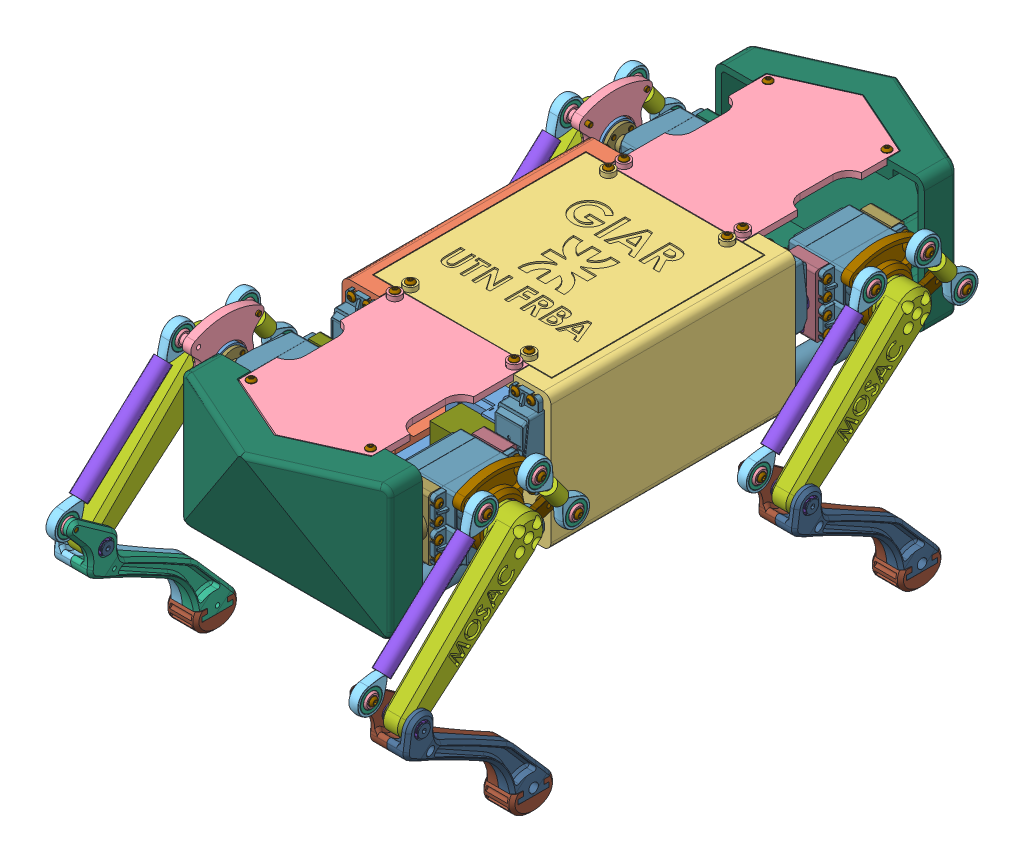
SolidWorks assembly Cuerpo_completo, configuration Default. Lengths in mm. (continued)
Components (placement in the parent): (continued)
- NUCLEO-F412ZG-3: NUCLEO-F412ZG [Default] at (0 3.6 5.7301) size (70 15.53 135.45)
- PCB_Interconexion-2: PCB_Interconexion [Default] at (-47.75 25.1914 50) x (1 0 0) z (0 1 0) size (106 111.32 17.03)
- IDC_40-1: IDC_40 [Default] at (-39.1382 -11.973 -4.2522) x (0 0 -1) z (1 0 0) size (55.48 10.75 7.86) (hidden)
- IDC_50-1: IDC_50 [Default] at (-15.8418 7.607 14.5537) x (0 0 1) z (-1 0 0) size (68.18 10.75 7.86) (hidden)
- IDC_50-2: IDC_50 [Default] at (45.1182 7.607 14.5537) x (0 0 1) z (-1 0 0) size (68.18 10.75 7.86) (hidden)
- IDC_50-4: IDC_50 [Default] at (4.87 250.7726 68.2196) x (0 0 -1) z (1 0 0) size (68.18 10.75 7.86) (hidden)
- IDC_50-5: IDC_50 [Default] at (-13.5299 250.7726 68.2196) x (0 0 -1) z (1 0 0) size (68.18 10.75 7.86) (hidden)
- IDC_40-2: IDC_40 [Default] at (-37.9534 250.7726 87.0269) x (0 0 1) z (-1 0 0) size (55.48 10.75 7.86) (hidden)
- USB-A-1: USB-A [Default] at (-40.9616 252.3756 123.8231) x (-1 0 0) z (0 0 -1) size (15 7 40) (hidden)
- USB-C-1: USB-C [Default] at (-43.6584 -12.82 23.9114) x (0 0 1) z (-1 0 0) size (10 5 29) (hidden)
- USB-C_90_Degree-1: USB-C_90_Degree [Default] at (31.45 -12.82 23.9114) x (0 0 -1) z (-1 0 0) size (25.07 7.5 16.55) (hidden)
- Tapa-1: Tapa [Default] at (0 39.5 0) size (114.5 7 136.5)
- Tapa_extrema-3: Tapa_extrema [Default] at (0 39.5 -161.6) x (1 0 0) z (0 1 0) size (85.5 120.4 7)
- Tapa_extrema-4: Tapa_extrema [Default] at (0.3648 39.5 161.4403) x (-0.999991 0 0.004156) z (0 1 0) size (85.5 120.4 7)
- Tornillo_boton_M3-1: Tornillo_boton_M3 [12] at (57.75 37.95 83.4927) x (0 0 -1) z (-1 -0.000079 0) size (13.65 5.5 5.5)
- Tornillo_boton_M3-2: Tornillo_boton_M3 [12] at (47.75 37.95 83.4927) x (0 0 -1) z (-0.987363 0.158475 0) size (13.65 5.5 5.5)
- Tornillo_boton_M3-4: Tornillo_boton_M3 [12] at (57.75 37.95 -83.4927) x (0 0 1) z (-0.423407 0.90594 0) size (13.65 5.5 5.5)
- Tornillo_boton_M3-6: Tornillo_boton_M3 [12] at (47.75 37.95 -83.4927) x (0 0 1) z (-0.25966 0.9657 0) size (13.65 5.5 5.5)
- Tornillo_boton_M3-8: Tornillo_boton_M3 [12] at (57.75 -11.55 83.4927) x (0 0 -1) z (-0.907023 0.421082 0) size (13.65 5.5 5.5)
- Tornillo_boton_M3-10: Tornillo_boton_M3 [12] at (47.75 -11.55 83.4927) x (0 0 -1) z (-0.902883 0.429885 0) size (13.65 5.5 5.5)
- Tornillo_boton_M3-12: Tornillo_boton_M3 [12] at (47.75 -11.55 -83.4927) x (0 0 1) z (0.257978 0.966151 0) size (13.65 5.5 5.5)
- Tornillo_boton_M3-14: Tornillo_boton_M3 [12] at (57.75 -11.55 -83.4927) x (0 0 1) z (0.421829 0.906675 0) size (13.65 5.5 5.5)
- Tornillo_boton_M3-16: Tornillo_boton_M3 [12] at (-47.75 -11.55 -83.4927) x (0 0 1) z (0.572863 0.819651 0) size (13.65 5.5 5.5)
- Tornillo_boton_M3-18: Tornillo_boton_M3 [12] at (-57.75 -11.55 -83.4927) x (0 0 1) z (0.706491 0.707722 0) size (13.65 5.5 5.5)
- Tornillo_boton_M3-20: Tornillo_boton_M3 [12] at (-47.75 37.95 -83.4927) x (0 0 1) z (0.818652 0.574289 0) size (13.65 5.5 5.5)
- Tornillo_boton_M3-22: Tornillo_boton_M3 [12] at (-57.75 37.95 -83.4927) x (0 0 1) z (0.90594 0.423407 0) size (13.65 5.5 5.5)
- Tornillo_boton_M3-24: Tornillo_boton_M3 [12] at (-47.75 37.95 83.4927) x (0 0 -1) z (-0.919584 -0.392893 0) size (13.65 5.5 5.5)
- Tornillo_boton_M3-26: Tornillo_boton_M3 [12] at (-57.75 37.95 83.4927) x (0 0 -1) z (-0.902816 -0.430028 0) size (13.65 5.5 5.5)
- Tornillo_boton_M3-28: Tornillo_boton_M3 [12] at (-47.75 -11.55 83.4927) x (0 0 -1) z (-0.906956 -0.421225 0) size (13.65 5.5 5.5)
- Tornillo_boton_M3-30: Tornillo_boton_M3 [12] at (-57.75 -11.55 83.4927) x (0 0 -1) z (-0.928542 -0.371227 0) size (13.65 5.5 5.5)
- Tornillo_boton_M3-31: Tornillo_boton_M3 [12] at (38.25 48.15 -63.75) x (0 -1 0) z (0.000424 0 1) size (13.65 5.5 5.5)
- Tornillo_boton_M3-32: Tornillo_boton_M3 [12] at (38.25 48.15 -73.75) x (0 -1 0) z (0.188872 0 0.982002) size (13.65 5.5 5.5)
- Tornillo_boton_M3-33: Tornillo_boton_M3 [12] at (-38.25 48.15 -63.75) x (0 -1 0) z (0.188872 0 0.982002) size (13.65 5.5 5.5)
- Tornillo_boton_M3-35: Tornillo_boton_M3 [12] at (-38.25 48.15 -73.75) x (0 -1 0) z (0.396124 0 0.918197) size (13.65 5.5 5.5)
- Tornillo_boton_M3-37: Tornillo_boton_M3 [12] at (-38.25 48.15 63.75) x (0 -1 0) z (0.600339 0 0.799745) size (13.65 5.5 5.5)
- Tornillo_boton_M3-39: Tornillo_boton_M3 [12] at (38.25 48.15 63.75) x (0 -1 0) z (0.773946 0 0.633251) size (13.65 5.5 5.5)
- Tornillo_boton_M3-41: Tornillo_boton_M3 [12] at (38.2493 48.15 73.4321) x (0 -1 0) z (0.896399 0 0.443249) size (13.65 5.5 5.5)
- Tornillo_boton_M3-43: Tornillo_boton_M3 [12] at (-38.25 48.15 73.75) x (0 -1 0) z (0.964846 0 0.262815) size (13.65 5.5 5.5)
- Tornillo_boton_M3-44: Tornillo_boton_M3 [12] at (-37.8641 45.15 166.5992) x (0 -1 0) z (0.997087 0 0.076276) size (13.65 5.5 5.5)
- Tornillo_boton_M3-46: Tornillo_boton_M3 [12] at (38.6352 45.15 166.2813) x (0 -1 0) z (0.990086 0 -0.140463) size (13.65 5.5 5.5)
- Tornillo_boton_M3-48: Tornillo_boton_M3 [12] at (-38.25 45.15 -166.6) x (0 -1 0) z (0.929566 0 -0.368656) size (13.65 5.5 5.5)
- Tornillo_boton_M3-50: Tornillo_boton_M3 [12] at (38.25 45.15 -166.6) x (0 -1 0) z (0.814641 0 -0.579966) size (13.65 5.5 5.5)
- Tornillo_boton_M3-52: Tornillo_boton_M3 [12] at (-38.25 -45.15 73.75) x (0 1 0) z (0.263634 0 0.964623) size (13.65 5.5 5.5)
- Tornillo_boton_M3-54: Tornillo_boton_M3 [12] at (38.25 -45.15 73.75) x (0 1 0) z (0.263634 0 0.964623) size (13.65 5.5 5.5)
- Tornillo_boton_M3-56: Tornillo_boton_M3 [12] at (38.25 -45.15 -73.75) x (0 1 0) z (0.263634 0 0.964623) size (13.65 5.5 5.5)
- Tornillo_boton_M3-58: Tornillo_boton_M3 [12] at (-38.25 -45.15 -73.75) x (0 1 0) z (0.263634 0 0.964623) size (13.65 5.5 5.5)
- Tornillo_PCB-1: Tornillo_PCB [Default] at (-24.5 -14.41 -26.3886) x (1 0 -0.000424) z (0.000424 0 1) size (6.68 7.05 6.27)
- Tornillo_PCB-2: Tornillo_PCB [Default] at (24.5 -14.41 -26.3886) x (0.982002 0 -0.188872) z (0.188872 0 0.982002) size (6.68 7.05 6.27)
- Tornillo_PCB-4: Tornillo_PCB [Default] at (24.5 -14.41 31.6114) x (0.918197 0 -0.396124) z (0.396124 0 0.918197) size (6.68 7.05 6.27)
- Tornillo_PCB-6: Tornillo_PCB [Default] at (-24.5 -14.41 31.6114) x (0.799745 0 -0.600339) z (0.600339 0 0.799745) size (6.68 7.05 6.27)
- Tornillo_PCB-8: Tornillo_PCB [Default] at (-24.13 5.18 -32.9499) x (0.672278 0 -0.740298) z (0.740298 0 0.672278) size (6.68 7.05 6.27)
- Tornillo_PCB-10: Tornillo_PCB [Default] at (8.89 5.18 19.1201) x (0.496883 0 -0.867817) z (0.867817 0 0.496883) size (6.68 7.05 6.27)
- Tornillo_PCB-12: Tornillo_PCB [Default] at (-42.75 25.1914 -45) x (0.982002 0 -0.188872) z (0.188872 0 0.982002) size (6.68 7.05 6.27)
- Tornillo_PCB-14: Tornillo_PCB [Default] at (53.25 25.1914 -45) x (0.918197 0 -0.396124) z (0.396124 0 0.918197) size (6.68 7.05 6.27)
- Tornillo_PCB-16: Tornillo_PCB [Default] at (53.25 25.1914 45) x (0.799745 0 -0.600339) z (0.600339 0 0.799745) size (6.68 7.05 6.27)
- Tornillo_PCB-18: Tornillo_PCB [Default] at (-42.75 25.1914 45) x (0.633251 0 -0.773946) z (0.773946 0 0.633251) size (6.68 7.05 6.27)
- Rocker Switch_KCD1-101_2pin-1: Rocker Switch_KCD1-101_2pin [Default] at (-67.25 23.9 0) x (0 0 1) z (-1 0 0) size (21.1 14.71 23.64)
- Stand-1: Stand [Default] at (0 -52.65 0) size (217.5 177.5 217.5) (hidden)
- Calibrator_Front-1: Calibrator_Front [Default] at (-96.75 2.8446 -78.75) x (0 0 1) z (-1 0 0) size (49.08 53.15 213.5) (hidden)
- Calibrator_Back-1: Calibrator_Back [Default] at (-96.25 2.4445 161.6) x (0 0 1) z (-1 0 0) size (141.93 52.75 212.5) (hidden)
Mates (geometry in assembly coordinates):
- Coincident7: coincident: line of Extremidad_FL-1/DS3235-3 through (-44.3004 33.1286 -78.75) axis (-1 0 0); plane of Lateral_left-1 through (-33.25 43.5 -78.75) normal (0 0 -1)
- Coincident17: coincident aligned: plane of Extremidad_FL-1/DS3235-3 through (-52.75 13.2 -71) normal (0 -1 0); plane of Lateral_left-1 through (-45.25 13.2 0) normal (0 -1 0)
- Concentric5: concentric aligned: cylinder of Extremidad_FL-1/DS3235-3 through (-57.75 37.95 -85.4) axis (0 0 -1) radius 2.25; cylinder of Lateral_left-1 through (-57.75 37.95 -66.75) axis (0 0 -1) radius 1.4
- Coincident10: coincident: line of Extremidad_BL-1/DS3235-3 through (-61.1996 33.1286 78.75) axis (1 0 0); plane of Lateral_left-1 through (-33.25 -43.5 78.75) normal (0 0 1)
- Coincident18: coincident aligned: plane of Extremidad_BL-1/DS3235-3 through (-52.75 13.2 71) normal (0 -1 0); plane of Lateral_left-1 through (-45.25 13.2 0) normal (0 -1 0)
- Concentric6: concentric aligned: cylinder of Extremidad_BL-1/DS3235-3 through (-57.75 37.95 85.4) axis (0 0 1) radius 2.25; cylinder of Lateral_left-1 through (-57.75 37.95 66.75) axis (0 0 1) radius 1.4
- Coincident19: coincident aligned: plane of Lateral_left-1 through (-33.25 43.5 -78.75) normal (0 0 -1); plane of Lateral_right-1 through (33.25 43.5 -78.75) normal (0 0 -1)
- Coincident20: coincident aligned: plane of Lateral_left-1 through (-33.25 43.5 78.75) normal (0 1 0); plane of Lateral_right-1 through (33.25 43.5 78.75) normal (0 1 0)
- Coincident21: coincident aligned: plane of Extremidad_FR-2/DS3235-3 through (52.75 13.2 -71) normal (0 -1 0); plane of Lateral_right-1 through (21.25 13.2 0) normal (0 -1 0)
- Coincident22: coincident: line of Extremidad_FR-2/DS3235-3 through (61.1996 33.1286 -78.75) axis (-1 0 0); plane of Lateral_right-1 through (33.25 43.5 -78.75) normal (0 0 -1)
- Concentric7: concentric aligned: cylinder of Extremidad_FR-2/DS3235-3 through (47.75 37.95 -85.4) axis (0 0 -1) radius 2.25; cylinder of Lateral_right-1 through (47.75 37.95 -66.75) axis (0 0 -1) radius 1.4
- Coincident23: coincident aligned: plane of Extremidad_BR-1/DS3235-3 through (52.75 13.2 71) normal (0 -1 0); plane of Lateral_right-1 through (21.25 13.2 0) normal (0 -1 0)
- Coincident24: coincident: line of Extremidad_BR-1/DS3235-3 through (44.3004 33.1286 78.75) axis (1 0 0); plane of Lateral_right-1 through (33.25 -43.5 78.75) normal (0 0 1)
- Concentric8: concentric aligned: cylinder of Extremidad_BR-1/DS3235-3 through (47.75 37.95 85.4) axis (0 0 1) radius 2.25; cylinder of Lateral_right-1 through (47.75 37.95 66.75) axis (0 0 1) radius 1.4
- Concentric9: concentric aligned: cylinder of Extremidad_BR-1/DS3235-3 through (57.75 37.95 85.4) axis (0 0 1) radius 2.25; cylinder of Tornillo_boton_M3-1 through (57.75 37.95 69.8427) axis (0 0 1) radius 1.5
- Coincident27: coincident: unknown of Extremidad_BR-1/DS3235-3; plane of Tornillo_boton_M3-1 through (57.7502 35.2 81.8427) normal (0 0 -1)
- Concentric10: concentric aligned: cylinder of Lateral_right-1 through (47.75 37.95 66.75) axis (0 0 1) radius 1.4; cylinder of Tornillo_boton_M3-2 through (47.75 37.95 69.8427) axis (0 0 1) radius 1.5
- Coincident29: coincident: unknown of Extremidad_BR-1/DS3235-3; plane of Tornillo_boton_M3-2 through (47.3142 35.2348 81.8427) normal (0 0 -1)
- Concentric11: concentric aligned: cylinder of Extremidad_FR-2/DS3235-3 through (57.75 37.95 -85.4) axis (0 0 -1) radius 2.25; cylinder of Tornillo_boton_M3-4 through (57.75 37.95 -69.8427) axis (0 0 -1) radius 1.5
- Coincident30: coincident: unknown of Extremidad_FR-2/DS3235-3; plane of Tornillo_boton_M3-4 through (60.2413 39.1144 -81.8427) normal (0 0 1)
- Concentric12: concentric aligned: cylinder of Lateral_right-1 through (47.75 37.95 -66.75) axis (0 0 -1) radius 1.4; cylinder of Tornillo_boton_M3-6 through (47.75 37.95 -69.8427) axis (0 0 -1) radius 1.5
- Coincident31: coincident: unknown of Extremidad_FR-2/DS3235-3; plane of Tornillo_boton_M3-6 through (50.4057 38.6641 -81.8427) normal (0 0 1)
- Concentric13: concentric aligned: cylinder of Tornillo_boton_M3-8 through (57.75 -11.55 69.8427) axis (0 0 1) radius 1.5; cylinder of Lateral_right-1 through (57.75 -11.55 66.75) axis (0 0 1) radius 1.4
- Coincident32: coincident: unknown of Extremidad_BR-1/DS3235-3; plane of Tornillo_boton_M3-8 through (56.592 -14.0443 81.8427) normal (0 0 -1)
- Concentric14: concentric aligned: cylinder of Lateral_right-1 through (47.75 -11.55 66.75) axis (0 0 1) radius 1.4; cylinder of Tornillo_boton_M3-10 through (47.75 -11.55 69.8427) axis (0 0 1) radius 1.5
- Coincident33: coincident: unknown of Extremidad_BR-1/DS3235-3; plane of Tornillo_boton_M3-10 through (46.5678 -14.0329 81.8427) normal (0 0 -1)
- Concentric15: concentric aligned: cylinder of Lateral_right-1 through (47.75 -11.55 -66.75) axis (0 0 -1) radius 1.4; cylinder of Tornillo_boton_M3-12 through (47.75 -11.55 -69.8427) axis (0 0 -1) radius 1.5
- Coincident34: coincident: unknown of Extremidad_FR-2/DS3235-3; plane of Tornillo_boton_M3-12 through (50.4069 -12.2594 -81.8427) normal (0 0 1)
- Concentric16: concentric aligned: cylinder of Extremidad_FR-2/DS3235-3 through (57.75 -11.55 -85.4) axis (0 0 -1) radius 2.25; cylinder of Tornillo_boton_M3-14 through (57.75 -11.55 -69.8427) axis (0 0 -1) radius 1.5
- Coincident35: coincident: unknown of Extremidad_FR-2/DS3235-3; plane of Tornillo_boton_M3-14 through (60.2434 -12.71 -81.8427) normal (0 0 1)
- Concentric17: concentric aligned: cylinder of Lateral_left-1 through (-47.75 -11.55 -66.75) axis (0 0 -1) radius 1.4; cylinder of Tornillo_boton_M3-16 through (-47.75 -11.55 -69.8427) axis (0 0 -1) radius 1.5
- Coincident36: coincident: unknown of Extremidad_FL-1/DS3235-3; plane of Tornillo_boton_M3-16 through (-45.496 -13.1254 -81.8427) normal (0 0 1)
- Concentric18: concentric aligned: cylinder of Lateral_left-1 through (-57.75 -11.55 -66.75) axis (0 0 -1) radius 1.4; cylinder of Tornillo_boton_M3-18 through (-57.75 -11.55 -69.8427) axis (0 0 -1) radius 1.5
- Coincident37: coincident: unknown of Extremidad_FL-1/DS3235-3; plane of Tornillo_boton_M3-18 through (-55.8038 -13.4929 -81.8427) normal (0 0 1)
- Concentric19: concentric aligned: cylinder of Lateral_left-1 through (-47.75 37.95 -66.75) axis (0 0 -1) radius 1.4; cylinder of Tornillo_boton_M3-20 through (-47.75 37.95 -69.8427) axis (0 0 -1) radius 1.5
- Coincident38: coincident: unknown of Extremidad_FL-1/DS3235-3; plane of Tornillo_boton_M3-20 through (-46.1707 35.6987 -81.8427) normal (0 0 1)
- Concentric20: concentric aligned: cylinder of Lateral_left-1 through (-57.75 37.95 -66.75) axis (0 0 -1) radius 1.4; cylinder of Tornillo_boton_M3-22 through (-57.75 37.95 -69.8427) axis (0 0 -1) radius 1.5
- Coincident39: coincident: unknown of Extremidad_FL-1/DS3235-3; plane of Tornillo_boton_M3-22 through (-56.5856 35.4587 -81.8427) normal (0 0 1)
- Concentric21: concentric aligned: cylinder of Lateral_left-1 through (-47.75 37.95 66.75) axis (0 0 1) radius 1.4; cylinder of Tornillo_boton_M3-24 through (-47.75 37.95 69.8427) axis (0 0 1) radius 1.5
- Coincident40: coincident: unknown of Extremidad_BL-1/DS3235-3; plane of Tornillo_boton_M3-24 through (-46.6695 35.4211 81.8427) normal (0 0 -1)
- Concentric22: concentric aligned: cylinder of Lateral_left-1 through (-57.75 37.95 66.75) axis (0 0 1) radius 1.4; cylinder of Tornillo_boton_M3-26 through (-57.75 37.95 69.8427) axis (0 0 1) radius 1.5
- Coincident41: coincident: unknown of Extremidad_BL-1/DS3235-3; plane of Tornillo_boton_M3-26 through (-56.5674 35.4673 81.8427) normal (0 0 -1)
- Concentric23: concentric aligned: cylinder of Lateral_left-1 through (-47.75 -11.55 66.75) axis (0 0 1) radius 1.4; cylinder of Tornillo_boton_M3-28 through (-47.75 -11.55 69.8427) axis (0 0 1) radius 1.5
- Coincident42: coincident: unknown of Extremidad_BL-1/DS3235-3; plane of Tornillo_boton_M3-28 through (-46.5916 -14.0441 81.8427) normal (0 0 -1)
- Concentric24: concentric aligned: cylinder of Lateral_left-1 through (-57.75 -11.55 66.75) axis (0 0 1) radius 1.4; cylinder of Tornillo_boton_M3-30 through (-57.75 -11.55 69.8427) axis (0 0 1) radius 1.5
- Coincident43: coincident: unknown of Extremidad_BL-1/DS3235-3; plane of Tornillo_boton_M3-30 through (-56.7291 -14.1035 81.8427) normal (0 0 -1)
- Concentric33: concentric aligned: cylinder of Varilla_hueca_aluminio-1 through (55.25 -31.5 2.5) axis (0 0 1) radius 8; cylinder of Lateral_right-1 through (55.25 -31.5 -22.6274) axis (0 0 1) radius 8
- Coincident52: coincident anti-aligned: plane of Lateral_right-1 through (45.25 0 2.5) normal (0 0 1); plane of Varilla_hueca_aluminio-1 through (55.25 -31.5 2.5) normal (0 0 -1)
- Concentric35: concentric aligned: cylinder of Lateral_right-1 through (55.25 -31.5 22.6274) axis (0 0 -1) radius 8; cylinder of Varilla_hueca_aluminio-4 through (55.25 -31.5 -2.5) axis (0 0 -1) radius 8
- Coincident54: coincident anti-aligned: plane of Lateral_right-1 through (45.25 0 -2.5) normal (0 0 -1); plane of Varilla_hueca_aluminio-4 through (55.25 -31.5 -2.5) normal (0 0 1)
- Concentric37: concentric aligned: cylinder of Lateral_left-1 through (-55.25 -31.5 22.6274) axis (0 0 -1) radius 8; cylinder of Varilla_hueca_aluminio-7 through (-55.25 -31.5 -2.5) axis (0 0 -1) radius 8
- Coincident57: coincident anti-aligned: plane of Lateral_left-1 through (-45.25 0 -2.5) normal (0 0 -1); plane of Varilla_hueca_aluminio-7 through (-55.25 -31.5 -2.5) normal (0 0 1)
- Coincident60: coincident anti-aligned: plane of Lateral_right-1 through (45.25 -39.5 0) normal (0 -1 0); plane of Base-1 through (0 -39.5 0) normal (0 1 0)
- Concentric38: concentric aligned: cylinder of Lateral_right-1 through (38.25 -43.501 73.75) axis (0 1 0) radius 2; cylinder of Base-1 through (38.25 -43.501 73.75) axis (0 1 0) radius 2
- Concentric39: concentric aligned: cylinder of Lateral_right-1 through (38.25 -43.501 -73.75) axis (0 1 0) radius 2; cylinder of Base-1 through (38.25 -43.501 -73.75) axis (0 1 0) radius 2
- Coincident49: coincident anti-aligned: plane of Base-1 through (0 -39.5 0) normal (0 1 0); plane of Battery-1 through (0 -39.5 0) normal (0 -1 0)
- Concentric46: concentric aligned: cylinder of Lateral_left-1 through (-55.25 -31.5 -22.6274) axis (0 0 1) radius 8; cylinder of Varilla_hueca_aluminio-2 through (-55.25 -31.5 2.5) axis (0 0 1) radius 8
- Coincident63: coincident anti-aligned: plane of Lateral_left-1 through (-45.25 0 2.5) normal (0 0 1); plane of Varilla_hueca_aluminio-2 through (-55.25 -31.5 2.5) normal (0 0 -1)
- Coincident71: coincident anti-aligned: plane of Lateral_right-1 through (45.25 39.5 0) normal (0 1 0); plane of Tapa-1 through (0 39.5 0) normal (0 -1 0)
- Concentric59: concentric aligned: cylinder of Lateral_right-1 through (38.25 43.501 63.75) axis (0 -1 0) radius 2; cylinder of Tapa-1 through (38.25 43.5 63.75) axis (0 -1 0) radius 2
- Coincident84: coincident anti-aligned: plane of Base-1 through (0 3.6 0) normal (0 1 0); plane of NUCLEO-F412ZG-3 through (-33 3.6 70.4001) normal (0 -1 0)
- Coincident74: coincident anti-aligned: plane of Battery-1 through (0 -39.5 0) normal (-1 0 0); plane of Base-1 through (0 -43.5 0) normal (1 0 0)
- Coincident75: coincident anti-aligned: plane of Battery-1 through (0 -39.5 0) normal (0 0 -1); plane of Base-1 through (0 -43.5 0) normal (0 0 1)
- Coincident83: coincident anti-aligned: plane of Base-1 through (0 -16 0) normal (0 1 0); plane of Raspberry Pi 4 Model B-2/PCB, RPi4ModelB-1 through (0 -16 -7.3886) normal (0 -1 0)
- Coincident85: coincident aligned: plane of Raspberry Pi 4 Model B-2 through (-24.5 -15.2 -7.3886) normal (-1 0 0); plane of IDC_40-1 through (-24.5 -11.973 -4.2522) normal (-1 0 0)
- Coincident86: coincident anti-aligned: plane of Raspberry Pi 4 Model B-2/2.54 mm DUPONT MALE PIN HEADER, IO, 2X20, RPi4ModelB-1 through (-25.77 -11.9 26.7414) normal (0 1 0); plane of IDC_40-1 through (-27.5 -11.9 -2.6686) normal (0 -1 0)
- Coincident87: coincident aligned: plane of Raspberry Pi 4 Model B-2 through (0 -15.2 2.6114) normal (0 0 -1); plane of IDC_40-1 through (-39.1382 -11.973 2.6114) normal (0 0 -1)
- Coincident88: coincident anti-aligned: plane of NUCLEO-F412ZG-3 through (-30.48 3.6 5.7301) normal (-1 0 0); plane of IDC_50-1 through (-30.48 7.607 14.5537) normal (1 0 0)
- Distance7: distance = 2.5 mm anti-aligned: plane of IDC_50-1 through (-27.48 7.68 12.9701) normal (0 -1 0); plane of NUCLEO-F412ZG-3 through (-33 5.18 70.4001) normal (0 1 0)
- Coincident90: coincident anti-aligned: plane of NUCLEO-F412ZG-3 through (0 3.6 -29.1399) normal (0 0 1); plane of IDC_50-1 through (-15.8418 7.607 -29.1399) normal (0 0 -1)
- Coincident91: coincident aligned: plane of NUCLEO-F412ZG-3 through (30.48 3.6 5.7301) normal (1 0 0); plane of IDC_50-2 through (30.48 7.607 14.5537) normal (1 0 0)
- Distance10: distance = 2.5 mm anti-aligned: plane of IDC_50-2 through (33.48 7.68 12.9701) normal (0 -1 0); plane of NUCLEO-F412ZG-3 through (-33 5.18 70.4001) normal (0 1 0)
- Coincident93: coincident anti-aligned: plane of NUCLEO-F412ZG-3 through (0 3.6 -29.1399) normal (0 0 1); plane of IDC_50-2 through (45.1182 7.607 -29.1399) normal (0 0 -1)
- Concentric60: concentric aligned: cylinder of Base-1 through (-24.13 -43.501 -32.9499) axis (0 1 0) radius 1.4; cylinder of NUCLEO-F412ZG-3 through (-24.13 0.353 -32.9499) axis (0 1 0) radius 1.6
- Concentric61: concentric aligned: cylinder of Base-1 through (8.89 -43.501 19.1201) axis (0 1 0) radius 1.4; cylinder of NUCLEO-F412ZG-3 through (8.89 0.353 19.1201) axis (0 1 0) radius 1.6
- Concentric62: concentric aligned: cylinder of Base-1 through (-24.5 -19.5 -26.3886) axis (0 1 0) radius 1.4; cylinder of Raspberry Pi 4 Model B-2/PCB, RPi4ModelB-1 through (-24.5 -14.4 -26.3886) axis (0 1 0) radius 1.35
- Concentric63: concentric aligned: cylinder of Base-1 through (24.5 -19.5 31.6114) axis (0 1 0) radius 1.4; cylinder of Raspberry Pi 4 Model B-2/PCB, RPi4ModelB-1 through (24.5 -14.4 31.6114) axis (0 1 0) radius 1.35
- Coincident110: coincident anti-aligned: plane of Varilla_hueca_aluminio-2 through (-55.25 -31.5 176.6) normal (0 0 1); plane of Extremo-1 through (-55.25 -31.5 176.6) normal (0 0 -1)
- Concentric78: concentric anti-aligned: cylinder of Varilla_hueca_aluminio-4 through (55.25 -31.5 -2.5) axis (0 0 -1) radius 8; cylinder of Extremo-2 through (55.25 -31.5 -176.6) axis (0 0 1) radius 8
- Coincident111: coincident anti-aligned: plane of Varilla_hueca_aluminio-4 through (55.25 -31.5 -176.6) normal (0 0 -1); plane of Extremo-2 through (55.25 -31.5 -176.6) normal (0 0 1)
- Coincident112: coincident anti-aligned: plane of Extremo-2 through (0 39.5 -211.6) normal (0 1 0); plane of Tapa_extrema-3 through (0 39.5 -161.6) normal (0 -1 0)
- Concentric79: concentric aligned: cylinder of Extremo-2 through (-38.25 43.501 -166.6) axis (0 -1 0) radius 2; cylinder of Tapa_extrema-3 through (-38.25 43.5 -166.6) axis (0 -1 0) radius 2
- Concentric80: concentric aligned: cylinder of Extremo-2 through (38.25 43.501 -166.6) axis (0 -1 0) radius 2; cylinder of Tapa_extrema-3 through (38.25 43.5 -166.6) axis (0 -1 0) radius 2
- Coincident113: coincident anti-aligned: plane of Extremo-1 through (0 39.5 211.6) normal (0 1 0); plane of Tapa_extrema-4 through (0.3648 39.5 161.4403) normal (0 -1 0)
- Concentric83: concentric anti-aligned: cylinder of Tapa-1 through (38.25 43.5 -63.75) axis (0 -1 0) radius 2; cylinder of Tornillo_boton_M3-31 through (38.25 34.5 -63.75) axis (0 1 0) radius 1.5
- Coincident114: coincident anti-aligned: plane of Tapa-1 through (38.25 46.5 -63.75) normal (0 1 0); plane of Tornillo_boton_M3-31 through (41 46.5 -63.7512) normal (0 -1 0)
- Concentric84: concentric anti-aligned: cylinder of Tapa_extrema-3 through (38.25 43.5 -73.75) axis (0 -1 0) radius 2; cylinder of Tornillo_boton_M3-32 through (38.25 34.5 -73.75) axis (0 1 0) radius 1.5
- Coincident122: coincident anti-aligned: plane of Tapa_extrema-3 through (38.25 46.5 -73.75) normal (0 1 0); plane of Tornillo_boton_M3-32 through (40.9505 46.5 -74.2694) normal (0 -1 0)
- Concentric85: concentric anti-aligned: cylinder of Tapa-1 through (-38.25 43.5 -63.75) axis (0 -1 0) radius 2; cylinder of Tornillo_boton_M3-33 through (-38.25 34.5 -63.75) axis (0 1 0) radius 1.5
- Coincident123: coincident anti-aligned: plane of Tapa-1 through (-38.25 46.5 -63.75) normal (0 1 0); plane of Tornillo_boton_M3-33 through (-35.5495 46.5 -64.2694) normal (0 -1 0)
- Concentric86: concentric anti-aligned: cylinder of Tapa_extrema-3 through (-38.25 43.5 -73.75) axis (0 -1 0) radius 2; cylinder of Tornillo_boton_M3-35 through (-38.25 34.5 -73.75) axis (0 1 0) radius 1.5
- Coincident124: coincident anti-aligned: plane of Tapa_extrema-3 through (-38.25 46.5 -73.75) normal (0 1 0); plane of Tornillo_boton_M3-35 through (-35.725 46.5 -74.8393) normal (0 -1 0)
- Concentric87: concentric anti-aligned: cylinder of Tapa-1 through (-38.25 43.5 63.75) axis (0 -1 0) radius 2; cylinder of Tornillo_boton_M3-37 through (-38.25 34.5 63.75) axis (0 1 0) radius 1.5
- Coincident125: coincident anti-aligned: plane of Tapa-1 through (-38.25 46.5 63.75) normal (0 1 0); plane of Tornillo_boton_M3-37 through (-36.0507 46.5 62.0991) normal (0 -1 0)
- Concentric88: concentric anti-aligned: cylinder of Tapa-1 through (38.25 43.5 63.75) axis (0 -1 0) radius 2; cylinder of Tornillo_boton_M3-39 through (38.25 34.5 63.75) axis (0 1 0) radius 1.5
- Coincident126: coincident anti-aligned: plane of Tapa-1 through (38.25 46.5 63.75) normal (0 1 0); plane of Tornillo_boton_M3-39 through (39.9914 46.5 61.6216) normal (0 -1 0)
- Concentric89: concentric anti-aligned: cylinder of Tapa_extrema-4 through (38.2493 43.5 73.4321) axis (0 -1 0) radius 2; cylinder of Tornillo_boton_M3-41 through (38.2493 34.5 73.4321) axis (0 1 0) radius 1.5
- Coincident127: coincident anti-aligned: plane of Tapa_extrema-4 through (38.2493 46.5 73.4321) normal (0 1 0); plane of Tornillo_boton_M3-41 through (39.4683 46.5 70.967) normal (0 -1 0)
- Concentric90: concentric anti-aligned: cylinder of Tapa_extrema-4 through (-38.25 43.5 73.75) axis (0 -1 0) radius 2; cylinder of Tornillo_boton_M3-43 through (-38.25 34.5 73.75) axis (0 1 0) radius 1.5
- Coincident128: coincident anti-aligned: plane of Tapa_extrema-4 through (-38.25 46.5 73.75) normal (0 1 0); plane of Tornillo_boton_M3-43 through (-37.5273 46.5 71.0967) normal (0 -1 0)
- Coincident130: coincident anti-aligned: plane of Lateral_left-1 through (-59.25 10.5 28.25) normal (1 0 0); plane of Buck-1 through (-59.25 0 0) normal (-1 0 0)
- Concentric91: concentric anti-aligned: cylinder of Lateral_left-1 through (-59.25 10.5 28.25) axis (-1 0 0) radius 1.4; cylinder of Buck-1 through (-57.65 10.5 28.25) axis (1 0 0) radius 1.25
- Concentric92: concentric anti-aligned: cylinder of Lateral_left-1 through (-59.25 -10.5 -28.25) axis (-1 0 0) radius 1.4; cylinder of Buck-1 through (-57.65 -10.5 -28.25) axis (1 0 0) radius 1.25
- Coincident131: coincident anti-aligned: plane of Raspberry Pi 4 Model B-2 through (0 -15.2 23.9114) normal (0 0 -1); plane of USB-C-1 through (-43.6584 -12.82 23.9114) normal (0 0 1)
- Coincident132: coincident aligned: plane of Raspberry Pi 4 Model B-2 through (0 -12.82 -7.3886) normal (0 1 0); plane of USB-C-1 through (-43.6584 -12.82 23.9114) normal (0 1 0)
- Coincident134: coincident aligned: plane of Raspberry Pi 4 Model B-2 through (0 -15.2 23.9114) normal (0 0 -1); plane of USB-C_90_Degree-1 through (31.45 -12.82 23.9114) normal (0 0 -1)
- Coincident135: coincident anti-aligned: plane of Raspberry Pi 4 Model B-2 through (0 -12.82 -7.3886) normal (0 1 0); plane of USB-C_90_Degree-1 through (31.45 -12.82 23.9114) normal (0 -1 0)
- Concentric93: concentric anti-aligned: cylinder of Tapa_extrema-4 through (-37.8641 43.5 166.5992) axis (0 -1 0) radius 2; cylinder of Tornillo_boton_M3-44 through (-37.8641 31.5 166.5992) axis (0 1 0) radius 1.5
- Coincident136: coincident anti-aligned: plane of Tapa_extrema-4 through (0.3648 43.5 161.4403) normal (0 1 0); plane of Tornillo_boton_M3-44 through (-37.6543 43.5 163.8572) normal (0 -1 0)
- Concentric94: concentric anti-aligned: cylinder of Tapa_extrema-4 through (38.6352 43.5 166.2813) axis (0 -1 0) radius 2; cylinder of Tornillo_boton_M3-46 through (38.6352 31.5 166.2813) axis (0 1 0) radius 1.5
- Coincident139: coincident anti-aligned: plane of Tapa_extrema-4 through (0.3648 43.5 161.4403) normal (0 1 0); plane of Tornillo_boton_M3-46 through (38.249 43.5 163.5585) normal (0 -1 0)
- Concentric95: concentric anti-aligned: cylinder of Tapa_extrema-3 through (-38.25 43.5 -166.6) axis (0 -1 0) radius 2; cylinder of Tornillo_boton_M3-48 through (-38.25 31.5 -166.6) axis (0 1 0) radius 1.5
- Coincident140: coincident anti-aligned: plane of Tapa_extrema-3 through (0 43.5 -161.6) normal (0 1 0); plane of Tornillo_boton_M3-48 through (-39.2638 43.5 -169.1563) normal (0 -1 0)
- Concentric96: concentric anti-aligned: cylinder of Tapa_extrema-3 through (38.25 43.5 -166.6) axis (0 -1 0) radius 2; cylinder of Tornillo_boton_M3-50 through (38.25 31.5 -166.6) axis (0 1 0) radius 1.5
- Coincident141: coincident anti-aligned: plane of Tapa_extrema-3 through (0 43.5 -161.6) normal (0 1 0); plane of Tornillo_boton_M3-50 through (36.6551 43.5 -168.8403) normal (0 -1 0)
- Concentric97: concentric anti-aligned: cylinder of Base-1 through (-38.25 -43.501 73.75) axis (0 1 0) radius 2; cylinder of Tornillo_boton_M3-52 through (-38.25 -31.5 73.75) axis (0 -1 0) radius 1.5
- Coincident142: coincident anti-aligned: plane of Base-1 through (0 -43.5 0) normal (0 -1 0); plane of Tornillo_boton_M3-52 through (-40.9027 -43.5 74.475) normal (0 1 0)
- Concentric98: concentric anti-aligned: cylinder of Base-1 through (38.25 -43.501 73.75) axis (0 1 0) radius 2; cylinder of Tornillo_boton_M3-54 through (38.25 -31.5 73.75) axis (0 -1 0) radius 1.5
- Coincident143: coincident anti-aligned: plane of Base-1 through (0 -43.5 0) normal (0 -1 0); plane of Tornillo_boton_M3-54 through (35.5973 -43.5 74.475) normal (0 1 0)
- Concentric99: concentric anti-aligned: cylinder of Base-1 through (38.25 -43.501 -73.75) axis (0 1 0) radius 2; cylinder of Tornillo_boton_M3-56 through (38.25 -31.5 -73.75) axis (0 -1 0) radius 1.5
- Coincident144: coincident anti-aligned: plane of Base-1 through (0 -43.5 0) normal (0 -1 0); plane of Tornillo_boton_M3-56 through (35.5973 -43.5 -73.025) normal (0 1 0)
- Concentric100: concentric anti-aligned: cylinder of Base-1 through (-38.25 -43.501 -73.75) axis (0 1 0) radius 2; cylinder of Tornillo_boton_M3-58 through (-38.25 -31.5 -73.75) axis (0 -1 0) radius 1.5
- Coincident145: coincident anti-aligned: plane of Base-1 through (0 -43.5 0) normal (0 -1 0); plane of Tornillo_boton_M3-58 through (-40.9027 -43.5 -73.025) normal (0 1 0)
- Coincident146: coincident anti-aligned: plane of Lateral_left-1 through (-45.25 23.5 0) normal (0 1 0); plane of PCB_Interconexion-2 through (5.25 23.5 0) normal (0 -1 0)
- Concentric101: concentric anti-aligned: cylinder of Lateral_left-1 through (-42.75 19.5 45) axis (0 1 0) radius 1.4; cylinder of PCB_Interconexion-2 through (-42.75 23.5 45) axis (0 -1 0) radius 1.75
- Concentric102: concentric anti-aligned: cylinder of Lateral_right-1 through (53.25 19.5 -45) axis (0 1 0) radius 1.4; cylinder of PCB_Interconexion-2 through (53.25 23.5 -45) axis (0 -1 0) radius 1.75
- Concentric103: concentric anti-aligned: cylinder of Varilla_hueca_aluminio-2 through (-55.25 -31.5 2.5) axis (0 0 1) radius 8; cylinder of Extremo-1 through (-55.25 -31.5 176.6) axis (0 0 -1) radius 8
- Concentric104: concentric anti-aligned: cylinder of Varilla_hueca_aluminio-1 through (55.25 -31.5 2.5) axis (0 0 1) radius 8; cylinder of Extremo-1 through (55.25 -31.5 176.6) axis (0 0 -1) radius 8
- Coincident147: coincident aligned: plane of Lateral_left-1 through (-67.25 0 0) normal (-1 0 0); plane of Rocker Switch_KCD1-101_2pin-1 through (-67.25 23.9 0) normal (-1 0 0)
- Coincident148: coincident aligned: plane of Lateral_left-1 through (-45.25 23.9 0) normal (0 1 0); plane of Rocker Switch_KCD1-101_2pin-1 through (-67.25 23.9 0) normal (0 1 0)
- Coincident149: coincident anti-aligned: plane of Lateral_left-1 through (-45.25 0 0) normal (0 0 -1); plane of Rocker Switch_KCD1-101_2pin-1 through (-67.25 23.9 0) normal (0 0 1)
- Concentric105: concentric aligned: cylinder of Base-1 through (-24.5 -19.5 -26.3886) axis (0 1 0) radius 1.4; cylinder of Tornillo_PCB-1 through (-24.5 -19.21 -26.3886) axis (0 1 0) radius 1.5
- Coincident150: coincident anti-aligned: plane of Raspberry Pi 4 Model B-2/PCB, RPi4ModelB-1 through (-24.5 -14.41 -26.3886) normal (0 1 0); plane of Tornillo_PCB-1 through (-24.5 -14.41 -26.3886) normal (0 -1 0)
- Concentric106: concentric aligned: cylinder of Base-1 through (24.5 -19.5 -26.3886) axis (0 1 0) radius 1.4; cylinder of Tornillo_PCB-2 through (24.5 -19.21 -26.3886) axis (0 1 0) radius 1.5
- Coincident151: coincident anti-aligned: plane of Raspberry Pi 4 Model B-2/PCB, RPi4ModelB-1 through (24.5 -14.41 -26.3886) normal (0 1 0); plane of Tornillo_PCB-2 through (24.5 -14.41 -26.3886) normal (0 -1 0)
- Concentric107: concentric aligned: cylinder of Base-1 through (24.5 -19.5 31.6114) axis (0 1 0) radius 1.4; cylinder of Tornillo_PCB-4 through (24.5 -19.21 31.6114) axis (0 1 0) radius 1.5
- Coincident152: coincident anti-aligned: plane of Raspberry Pi 4 Model B-2/PCB, RPi4ModelB-1 through (24.5 -14.41 31.6114) normal (0 1 0); plane of Tornillo_PCB-4 through (24.5 -14.41 31.6114) normal (0 -1 0)
- Concentric108: concentric aligned: cylinder of Base-1 through (-24.5 -19.5 31.6114) axis (0 1 0) radius 1.4; cylinder of Tornillo_PCB-6 through (-24.5 -19.21 31.6114) axis (0 1 0) radius 1.5
- Coincident153: coincident anti-aligned: plane of Raspberry Pi 4 Model B-2/PCB, RPi4ModelB-1 through (-24.5 -14.41 31.6114) normal (0 1 0); plane of Tornillo_PCB-6 through (-24.5 -14.41 31.6114) normal (0 -1 0)
- Concentric109: concentric aligned: cylinder of Base-1 through (-24.13 -43.501 -32.9499) axis (0 1 0) radius 1.4; cylinder of Tornillo_PCB-8 through (-24.13 0.38 -32.9499) axis (0 1 0) radius 1.5
- Coincident154: coincident anti-aligned: plane of NUCLEO-F412ZG-3 through (-33 5.18 70.4001) normal (0 1 0); plane of Tornillo_PCB-8 through (-24.13 5.18 -32.9499) normal (0 -1 0)
- Concentric110: concentric aligned: cylinder of Base-1 through (8.89 -43.501 19.1201) axis (0 1 0) radius 1.4; cylinder of Tornillo_PCB-10 through (8.89 0.38 19.1201) axis (0 1 0) radius 1.5
- Coincident155: coincident anti-aligned: plane of NUCLEO-F412ZG-3 through (-33 5.18 70.4001) normal (0 1 0); plane of Tornillo_PCB-10 through (8.89 5.18 19.1201) normal (0 -1 0)
- Concentric111: concentric aligned: cylinder of Lateral_left-1 through (-42.75 19.5 -45) axis (0 1 0) radius 1.4; cylinder of Tornillo_PCB-12 through (-42.75 20.3914 -45) axis (0 1 0) radius 1.5
- Coincident156: coincident anti-aligned: plane of PCB_Interconexion-2 through (5.25 25.1914 0) normal (0 1 0); plane of Tornillo_PCB-12 through (-42.75 25.1914 -45) normal (0 -1 0)
- Concentric112: concentric aligned: cylinder of Lateral_right-1 through (53.25 19.5 -45) axis (0 1 0) radius 1.4; cylinder of Tornillo_PCB-14 through (53.25 20.3914 -45) axis (0 1 0) radius 1.5
- Coincident157: coincident anti-aligned: plane of PCB_Interconexion-2 through (5.25 25.1914 0) normal (0 1 0); plane of Tornillo_PCB-14 through (53.25 25.1914 -45) normal (0 -1 0)
- Concentric113: concentric aligned: cylinder of Lateral_right-1 through (53.25 19.5 45) axis (0 1 0) radius 1.4; cylinder of Tornillo_PCB-16 through (53.25 20.3914 45) axis (0 1 0) radius 1.5
- Coincident158: coincident anti-aligned: plane of PCB_Interconexion-2 through (5.25 25.1914 0) normal (0 1 0); plane of Tornillo_PCB-16 through (53.25 25.1914 45) normal (0 -1 0)
- Concentric114: concentric aligned: cylinder of Lateral_left-1 through (-42.75 19.5 45) axis (0 1 0) radius 1.4; cylinder of Tornillo_PCB-18 through (-42.75 20.3914 45) axis (0 1 0) radius 1.5
- Coincident159: coincident anti-aligned: plane of PCB_Interconexion-2 through (5.25 25.1914 0) normal (0 1 0); plane of Tornillo_PCB-18 through (-42.75 25.1914 45) normal (0 -1 0)
- Coincident160: coincident anti-aligned: plane of Raspberry Pi 4 Model B-2/Female USB Type C Connector, RPi4ModelB-1 through (24.8 -12.82 23.9114) normal (1 0 0); plane of USB-C_90_Degree-1 through (24.8 -11.62 26.8614) normal (-1 0 0)
- Tangent2: tangent aligned: cylinder of Tornillo_boton_M3-46 through (38.6352 31.5 166.2813) axis (0 1 0) radius 1.5; cylinder of Extremo-1 through (38.25 43.501 166.6) axis (0 -1 0) radius 2
- Concentric115: concentric anti-aligned: cylinder of Lateral_left-1 through (-38.25 43.501 -63.75) axis (0 -1 0) radius 2; cylinder of Tornillo_boton_M3-33 through (-38.25 34.5 -63.75) axis (0 1 0) radius 1.5
- Concentric116: concentric anti-aligned: cylinder of Varilla_hueca_aluminio-7 through (-55.25 -31.5 -2.5) axis (0 0 -1) radius 8; cylinder of Extremo-2 through (-55.25 -31.5 -176.6) axis (0 0 1) radius 8
- Concentric117: concentric anti-aligned: cylinder of Lateral_left-1 through (-38.25 43.501 73.75) axis (0 -1 0) radius 2; cylinder of Tornillo_boton_M3-43 through (-38.25 34.5 73.75) axis (0 1 0) radius 1.5
- Coincident162: coincident: plane of Tapa-1 through (0 39.5 0) normal (0 0 1)
- Coincident163: coincident: plane of Tapa-1 through (0 39.5 0) normal (1 0 0)
- Coincident164: coincident: plane of Lateral_right-1 through (21.25 0 0) normal (0 1 0)
- Coincident165: coincident aligned: plane of Tapa-1 through (0 39.5 0) normal (0 0 1)
- Coincident166: coincident aligned: plane of Tapa-1 through (0 39.5 0) normal (1 0 0)
- Coincident167: coincident anti-aligned: plane of Tornillo_boton_M3-52 through (-38.25 -45.15 73.75) normal (0 -1 0); plane of Stand-1 through (0 -45.15 0) normal (0 1 0)
- Coincident168: coincident aligned: plane of Stand-1 through (0 -52.65 0) normal (1 0 0)
- Coincident169: coincident aligned: plane of Stand-1 through (0 -52.65 0) normal (0 0 1)
- Distance12: distance = 0.5 mm anti-aligned: plane of Lateral_left-1 through (-67.25 0 0) normal (-1 0 0); plane of Calibrator_Front-1 through (-67.75 2.8446 -78.75) normal (1 0 0)
- Coincident176: coincident anti-aligned: plane of Lateral_left-1 through (-33.25 -43.5 -78.75) normal (0 -1 0); plane of Calibrator_Front-1 through (-55.75 -43.5 -78.75) normal (0 1 0)
- Coincident177: coincident anti-aligned: plane of Lateral_left-1 through (-33.25 43.5 -78.75) normal (0 0 -1); plane of Calibrator_Front-1 through (-55.75 2.8446 -78.75) normal (0 0 1)
- Distance13: distance = 0.5 mm anti-aligned: plane of Extremo-1 through (-67.25 -43.5 161.6) normal (-1 0 0); plane of Calibrator_Back-1 through (-67.75 2.4445 161.6) normal (1 0 0)
- Coincident179: coincident anti-aligned: plane of Extremo-1 through (0 0 161.6) normal (0 0 -1); plane of Calibrator_Back-1 through (-55.25 2.4445 161.6) normal (0 0 1)
- Coincident180: coincident anti-aligned: plane of Extremo-1 through (67.25 -43.5 161.6) normal (0 -1 0); plane of Calibrator_Back-1 through (-55.25 -43.5 161.6) normal (0 1 0)
